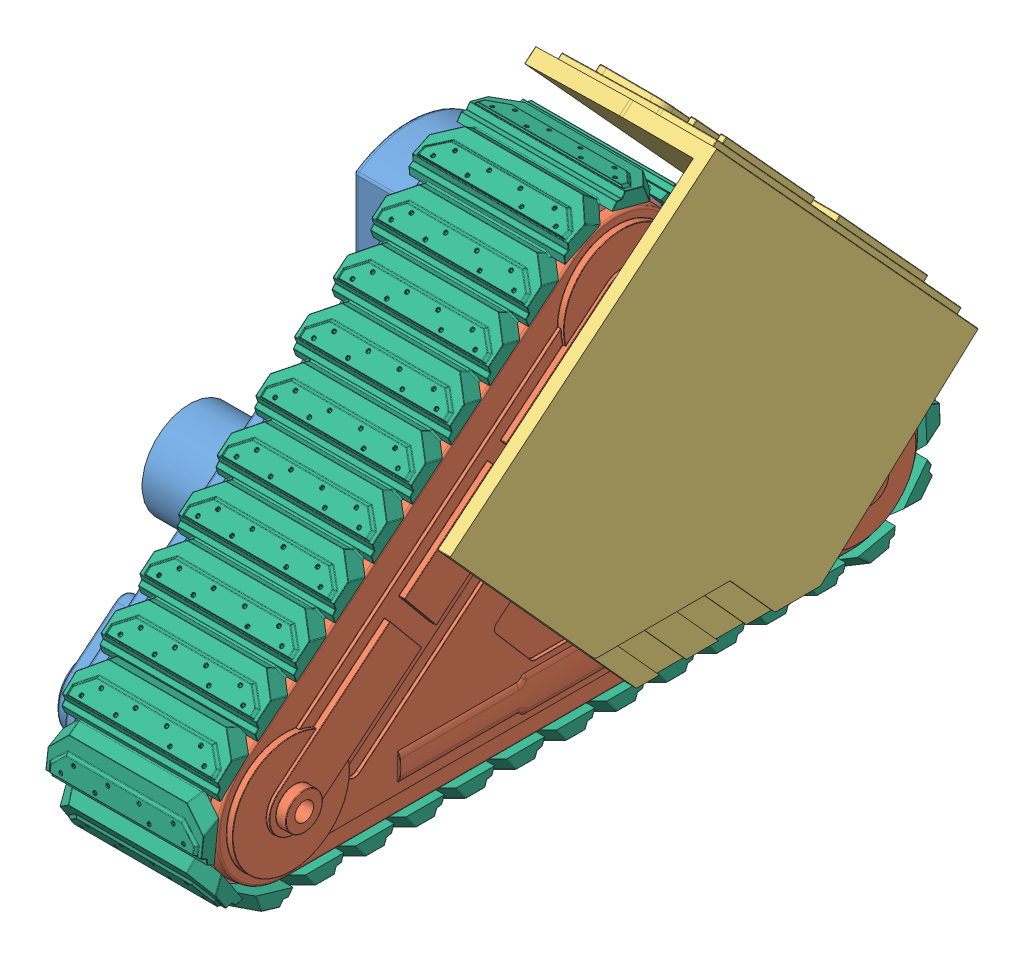
SolidWorks assembly TDRV (Left), configuration Default. Lengths in mm.
Overall size (51.05 82.74 123.21).
17 component instances, 8 part files, 34 mates.
Components (placement in the parent):
- Track Drive Side (Left, Inner)-1: Track Drive Side (Left, Inner) [Default] at (-11.975 -11 -45.5) size (22.2 65.97 113)
- Track Drive Side (Left, Outer)-1: Track Drive Side (Left, Outer) [Default] at (11.975 -11 -45.5) size (26.75 65.97 113)
- TDRV Beauty Cover (Left)-1: TDRV Beauty Cover (Left) [Default] at (20.575 -4.6199 -48.4187) x (1 0 0) z (0 -0.001763 0.999998) size (32.9 69.17 84.78)
- Roller-1: Roller [Default] x (1 0 0) z (0 -0.637242 0.770664) size (18.92 25.7 25.7)
  - Roller (Female)-1: Roller (Female) [Default] at (5.16 0 0) size (10.22 25.7 25.7)
  - Roller (Male)-1: Roller (Male) [Default] at (-5.16 0 0) size (13 25.7 25.7)
- Roller-2: Roller [Default] at (0 0 -91) x (1 0 0) z (0 1 0) size (18.92 25.7 25.7)
  - Roller (Female)-1: Roller (Female) [Default] at (5.16 0 0) size (10.22 25.7 25.7)
  - Roller (Male)-1: Roller (Male) [Default] at (-5.16 0 0) size (13 25.7 25.7)
- Roller-3: Roller [Default] at (0 43.9697 -53.1758) x (1 0 0) z (0 -0.637242 0.770664) size (18.92 25.7 25.7)
  - Roller (Female)-1: Roller (Female) [Default] at (5.16 0 0) size (10.22 25.7 25.7)
  - Roller (Male)-1: Roller (Male) [Default] at (-5.16 0 0) size (13 25.7 25.7)
- Treads-1: Treads [Default] at (0 -11 -45.5) size (25 72.41 119.4)
- Cheese Head Thread-Forming Screw 2.8mm x 8mm-1: Cheese Head Thread-Forming Screw 2.8mm x 8mm [Default] at (-4.275 0 0) x (0 1 0) z (0 0 1) size (5.45 9.97 5.45)
- Cheese Head Thread-Forming Screw 2.8mm x 8mm-3: Cheese Head Thread-Forming Screw 2.8mm x 8mm [Default] at (-4.275 0 -91) x (0 1 0) z (0 0 1) size (5.45 9.97 5.45)
- Cheese Head Thread-Forming Screw 2.8mm x 8mm-7: Cheese Head Thread-Forming Screw 2.8mm x 8mm [Default] at (-4.275 43.9697 -53.1758) x (0 -1 0) z (0 0 -1) size (5.45 9.97 5.45)
- Washer Head Thread-Forming Screw 2.6mm x 6mm-1: Washer Head Thread-Forming Screw 2.6mm x 6mm [Default] at (-18.575 36.4697 -53.1758) x (0 1 0) z (0 0 1) size (7.8 7.44 7.8)
Mates (geometry in assembly coordinates):
- Concentric17: concentric aligned: cylinder of Track Drive Side (Left, Inner)-1 through (-11.975 0 0) axis (1 0 0) radius 1.7; cylinder of Track Drive Side (Left, Outer)-1 through (-39.5931 0 0) axis (1 0 0) radius 3.1
- Coincident17: coincident anti-aligned: plane of Track Drive Side (Left, Inner)-1 through (-10.275 -11 -45.5) normal (1 0 0); plane of Track Drive Side (Left, Outer)-1 through (-10.275 -11 -45.5) normal (-1 0 0)
- Concentric18: concentric aligned: cylinder of Track Drive Side (Left, Inner)-1 through (-11.975 0 -91) axis (1 0 0) radius 1.7; cylinder of Track Drive Side (Left, Outer)-1 through (-39.5931 0 -91) axis (1 0 0) radius 3.1
- Concentric19: concentric: cylinder of Track Drive Side (Left, Inner)-1 through (-44.8171 0 0) axis (1 0 0) radius 3.525; point of assembly
- Parallel5: parallel aligned: plane of Track Drive Side (Left, Inner)-1 through (-11.975 -11 -45.5) normal (0 1 0); plane of assembly through (0 0 0) normal (0 1 0)
- Symmetric2: symmetric aligned: plane of Track Drive Side (Left, Inner)-1 through (-11.975 -11 -45.5) normal (-1 0 0); plane of Track Drive Side (Left, Outer)-1 through (11.975 -11 -45.5) normal (1 0 0); plane of assembly through (0 0 0) normal (1 0 0)
- Concentric1: concentric aligned: cylinder of Track Drive Side (Left, Inner)-1 through (-11.975 0 0) axis (1 0 0) radius 1.7; cylinder of Roller-1/Roller (Male)-1 through (-9.46 0 0) axis (1 0 0) radius 3.5
- Concentric2: concentric aligned: cylinder of Track Drive Side (Left, Inner)-1 through (-11.975 0 -91) axis (1 0 0) radius 1.7; cylinder of Roller-2/Roller (Male)-1 through (-9.46 0 -91) axis (1 0 0) radius 3.5
- Concentric3: concentric aligned: cylinder of Track Drive Side (Left, Inner)-1 through (-11.975 43.9697 -53.1758) axis (1 0 0) radius 1.7; cylinder of Roller-3/Roller (Male)-1 through (-9.46 43.9697 -53.1758) axis (1 0 0) radius 3.5
- Symmetric1: symmetric aligned: plane of Track Drive Side (Left, Inner)-1 through (-11.975 -11 -45.5) normal (-1 0 0); plane of Track Drive Side (Left, Outer)-1 through (11.975 -11 -45.5) normal (1 0 0); plane of assembly through (0 0 0) normal (1 0 0)
- Coincident2: coincident aligned: plane of Roller-1; plane of assembly through (0 0 0) normal (1 0 0)
- Coincident3: coincident aligned: plane of Roller-1; plane of Roller-2
- Coincident4: coincident aligned: plane of Roller-1; plane of Roller-3
- Coincident5: coincident anti-aligned: plane of Track Drive Side (Left, Outer)-1 through (16.475 12.3697 -42.5013) normal (1 0 0); plane of TDRV Beauty Cover (Left)-1 through (16.475 -4.6199 -48.4187) normal (-1 0 0)
- Concentric4: concentric aligned: cylinder of Track Drive Side (Left, Outer)-1 through (-10.275 12.3697 -42.5013) axis (1 0 0) radius 1.6; cylinder of TDRV Beauty Cover (Left)-1 through (-1.2676 12.3697 -42.5013) axis (1 0 0) radius 1.5
- Concentric5: concentric aligned: cylinder of Track Drive Side (Left, Outer)-1 through (-10.275 24 -75.088) axis (1 0 0) radius 1.6; cylinder of TDRV Beauty Cover (Left)-1 through (-1.2676 24 -75.088) axis (1 0 0) radius 1.5
- Concentric6: concentric aligned: cylinder of Track Drive Side (Left, Inner)-1 through (-23.675 36.4697 -53.1758) axis (-1 0 0) radius 0.8; cylinder of Washer Head Thread-Forming Screw 2.6mm x 6mm-1 through (-25.975 36.4697 -53.1758) axis (-1 0 0) radius 1.3
- Distance1: distance = 2.9 mm anti-aligned: plane of Washer Head Thread-Forming Screw 2.6mm x 6mm-1 through (-24.375 35.1697 -53.1758) normal (1 0 0); plane of Track Drive Side (Left, Inner)-1 through (-21.475 -11 -45.5) normal (-1 0 0)
- Parallel1: parallel aligned: plane of Washer Head Thread-Forming Screw 2.6mm x 6mm-1; plane of assembly through (0 0 0) normal (0 1 0)
- Concentric7: concentric aligned: cylinder of Track Drive Side (Left, Outer)-1 through (-10.275 0 0) axis (-1 0 0) radius 0.9; cylinder of Cheese Head Thread-Forming Screw 2.8mm x 8mm-1 through (-14.175 0 0) axis (-1 0 0) radius 1.4
- Parallel4: parallel aligned: plane of Cheese Head Thread-Forming Screw 2.8mm x 8mm-1; plane of assembly through (0 0 0) normal (0 1 0)
- Coincident7: coincident anti-aligned: plane of Track Drive Side (Left, Inner)-1 through (-11.975 -11 -45.5) normal (-1 0 0); plane of Cheese Head Thread-Forming Screw 2.8mm x 8mm-1 through (-11.975 -1.4 0) normal (1 0 0)
- Parallel3: parallel aligned: plane of Cheese Head Thread-Forming Screw 2.8mm x 8mm-3; plane of assembly through (0 0 0) normal (0 1 0)
- Concentric10: concentric aligned: cylinder of Track Drive Side (Left, Outer)-1 through (-10.275 0 -91) axis (-1 0 0) radius 0.9; cylinder of Cheese Head Thread-Forming Screw 2.8mm x 8mm-3 through (-14.175 0 -91) axis (-1 0 0) radius 1.4
- Coincident10: coincident anti-aligned: plane of Track Drive Side (Left, Inner)-1 through (-11.975 -11 -45.5) normal (-1 0 0); plane of Cheese Head Thread-Forming Screw 2.8mm x 8mm-3 through (-11.975 -1.4 -91) normal (1 0 0)
- Concentric16: concentric aligned: cylinder of Track Drive Side (Left, Outer)-1 through (-10.275 43.9697 -53.1758) axis (-1 0 0) radius 0.9; cylinder of Cheese Head Thread-Forming Screw 2.8mm x 8mm-7 through (-14.175 43.9697 -53.1758) axis (-1 0 0) radius 1.4
- Parallel2: parallel anti-aligned: plane of Cheese Head Thread-Forming Screw 2.8mm x 8mm-7; plane of assembly through (0 0 0) normal (0 1 0)
- Coincident16: coincident anti-aligned: plane of Track Drive Side (Left, Inner)-1 through (-11.975 -11 -45.5) normal (-1 0 0); plane of Cheese Head Thread-Forming Screw 2.8mm x 8mm-7 through (-11.975 45.3697 -53.1758) normal (1 0 0)
- Coincident18: coincident aligned: plane of Treads-1 through (0 -11 -45.5) normal (1 0 0); plane of assembly through (0 0 0) normal (1 0 0)
- Concentric20: concentric aligned: cylinder of Track Drive Side (Left, Inner)-1 through (-44.8171 0 0) axis (1 0 0) radius 3.525; circle of Treads-1
- Concentric21: concentric aligned: cylinder of Track Drive Side (Left, Inner)-1 through (-32.5371 0 -91) axis (1 0 0) radius 3.525; circle of Treads-1
- Parallel6: parallel aligned: plane of Track Drive Side (Left, Outer)-1 through (54.164 20.9608 -19.0724) normal (0 0.770664 0.637242); plane of Roller-1 through (0 0 0) normal (0 0.770664 0.637242)
- Parallel7: parallel aligned: plane of Roller-2 through (0 0 -91) normal (0 1 0); plane of assembly through (0 0 0) normal (0 1 0)
- Parallel8: parallel aligned: plane of Track Drive Side (Left, Outer)-1 through (54.164 20.9608 -19.0724) normal (0 0.770664 0.637242); plane of Roller-3 through (0 43.9697 -53.1758) normal (0 0.770664 0.637242)
